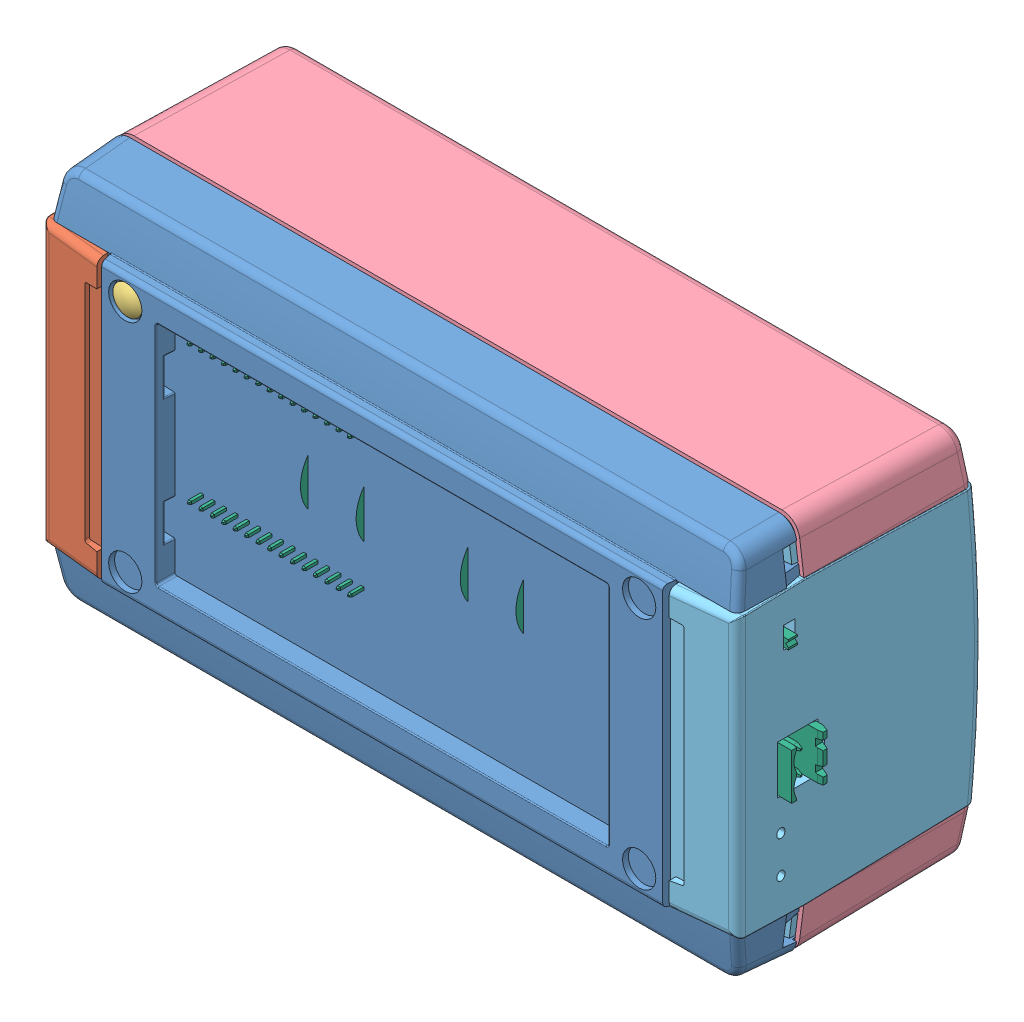
SolidWorks assembly Assembly, configuration Default. Lengths in mm.
Overall size (160.27 84 56.92).
19 component instances, 12 part files, 12 mates.
Components (placement in the parent):
- B1060365 154_84_56-1: B1060365 154_84_56 [Default] at (1.25 0 -12.8) x (0 1 0) z (-1 0 0) size (84 72.92 156.75)
  - 00007483 - 154 Unterteil-1: 00007483 - 154 Unterteil [Default] x (-1 0 0) z (0 0 -1) size (84 17.8 153.5)
  - 00007882 - Gummifuss  D6,5 x 2 mm-1: 00007882 - Gummifuss  D6,5 x 2 mm [Default] at (26 -15.6 -57) x (0.536953 0 0.843612) z (0.843612 0 -0.536953) size (6.6 2.04 6.75) (hidden)
  - 00006113 - 154 Stirnteil H ohne Lⁿftung-5: 00006113 - 154 Stirnteil H ohne Lⁿftung [Default] at (0 -16.8 63.3) x (0 0 1) z (-1 0 0) size (15.5 56 77)
  - 00007882 - Gummifuss  D6,5 x 2 mm-2: 00007882 - Gummifuss  D6,5 x 2 mm [Default] at (26 -15.6 57) x (0.536953 0 0.843612) z (0.843612 0 -0.536953) size (6.6 2.04 6.75)
  - 00007882 - Gummifuss  D6,5 x 2 mm-3: 00007882 - Gummifuss  D6,5 x 2 mm [Default] at (-26 -15.6 57) x (-0.536953 0 -0.843612) z (-0.843612 0 0.536953) size (6.6 2.04 6.75) (hidden)
  - 00006613 - Wandhalter 154_Default-1: 00006613 - Wandhalter 154_Default [Default] at (0 -12.8 1.25) x (0 0 -1) z (0 -1 0) size (133 49.6 8) (hidden)
  - 00007733 - Rastfuss-1: 00007733 - Rastfuss [Default] at (0 -15 38) x (-1 0 0) z (0 0 1) size (11.01 20.6 76) (hidden)
  - 00007864 - Liko-Schraube 2.5x6 Arnold Plastide 45 KS Z (PZ1) blau verz.-1: 00007864 - Liko-Schraube 2.5x6 Arnold Plastide 45 KS Z (PZ1) blau verz. [Default] at (-31.5 -4.7 -58) size (4 7.8 4) (hidden)
  - 00007864 - Liko-Schraube 2.5x6 Arnold Plastide 45 KS Z (PZ1) blau verz.-2: 00007864 - Liko-Schraube 2.5x6 Arnold Plastide 45 KS Z (PZ1) blau verz. [Default] at (29 -4.7 58) x (-1 0 0) z (0 0 -1) size (4 7.8 4) (hidden)
  - 00007864 - Liko-Schraube 2.5x6 Arnold Plastide 45 KS Z (PZ1) blau verz.-3: 00007864 - Liko-Schraube 2.5x6 Arnold Plastide 45 KS Z (PZ1) blau verz. [Default] at (-29 -4.7 58) size (4 7.8 4) (hidden)
  - 00007864 - Liko-Schraube 2.5x6 Arnold Plastide 45 KS Z (PZ1) blau verz.-4: 00007864 - Liko-Schraube 2.5x6 Arnold Plastide 45 KS Z (PZ1) blau verz. [Default] at (31.5 -4.7 -58) x (-1 0 0) z (0 0 -1) size (4 7.8 4) (hidden)
  - 00007482 - 154 Oberteil H-1: 00007482 - 154 Oberteil H [Default] at origin size (84 37.76 153.73)
  - 00007882 - Gummifuss  D6,5 x 2 mm-4: 00007882 - Gummifuss  D6,5 x 2 mm [Default] at (-26 -15.6 -57) x (-0.536953 0 -0.843612) z (-0.843612 0 0.536953) size (6.6 2.04 6.75) (hidden)
  - 00006113 - 156 Stirnteil H ohne Lⁿftung-1: 00006113 - 156 Stirnteil H ohne Lⁿftung [Default] at (0 -16.4764 -63.3454) x (0 0 -1) z (1 0 0) size (15.5 56 77)
- PCB5_Altuim-1: PCB5_Altuim [Default] at (-71.752 -153.051 -18.1194) x (0 1 0) z (0 0 -1) size (75.03 156.42 35.06) (hidden)
- PCB6_Altuim-1: PCB6_Altuim [Default] at (-100.403 -65.036 -16.9115) x (0 1 0) z (0 0 -1) size (75.18 156.42 35.06) (hidden)
- PCB_Voltix_v8.4-1: PCB_Voltix_v8.4 [Défaut] at (-99.49 -65.036 -6.9115) x (0 1 0) z (0 0 -1) size (75.16 160.27 34.6)
- Ledss-1: Ledss [Défaut] at (51.0563 -24.9243 -6.9115) x (0 1 0) z (0 0 -1) size (4 11.76 39.59)
Mates (geometry in assembly coordinates):
- Coincident1: coordinate: point of B1060365 154_84_56-1/00006613 - Wandhalter 154_Default-1; point of assembly
- Concentric12: concentric anti-aligned: cylinder of B1060365 154_84_56-1/00007864 - Liko-Schraube 2.5x6 Arnold Plastide 45 KS Z (PZ1) blau verz.-4 through (59.25 31.5 -2.1) axis (0 0 -1) radius 1.25; cylinder of PCB5_Altuim-1 through (59.25 31.5 -16.5) axis (0 0 1) radius 1.5
- Parallel6: parallel anti-aligned: plane of B1060365 154_84_56-1/00006113 - 156 Stirnteil H ohne Lⁿftung-1 through (75.7954 0 247.6764) normal (-1 0 0); plane of PCB5_Altuim-1 through (74.704 -13.726 -16.5) normal (1 0 0)
- Distance3: distance = 10 mm anti-aligned: plane of B1060365 154_84_56-1/00007483 - 154 Unterteil-1 through (59.25 31.5 -6.5) normal (0 0 -1); plane of PCB6_Altuim-1 through (1.2255 -0.1709 -16.5) normal (0 0 1)
- Concentric13: concentric anti-aligned: cylinder of B1060365 154_84_56-1/00007864 - Liko-Schraube 2.5x6 Arnold Plastide 45 KS Z (PZ1) blau verz.-4 through (59.25 31.5 -2.1) axis (0 0 -1) radius 1.25; cylinder of PCB6_Altuim-1 through (59.25 31.5 -16.5) axis (0 0 1) radius 1.5
- Parallel7: parallel anti-aligned: plane of B1060365 154_84_56-1/00006113 - 156 Stirnteil H ohne Lⁿftung-1 through (75.7954 0 247.6764) normal (-1 0 0); plane of PCB6_Altuim-1 through (74.73 -13.243 -16.5) normal (1 0 0)
- Distance4: distance = 0 mm anti-aligned: plane of B1060365 154_84_56-1/00007483 - 154 Unterteil-1 through (-56.75 29 -6.5) normal (0 0 -1); plane of PCB_Voltix_v8.4-1 through (1.2185 -0.1501 -6.5) normal (0 0 1)
- Parallèle1: parallel anti-aligned: plane of B1060365 154_84_56-1/00006113 - 156 Stirnteil H ohne Lⁿftung-1 through (75.7954 0 247.6764) normal (-1 0 0); plane of PCB_Voltix_v8.4-1 through (74.73 -13.144 -6.5) normal (1 0 0)
- Coaxiale1: concentric anti-aligned: cylinder of B1060365 154_84_56-1/00007864 - Liko-Schraube 2.5x6 Arnold Plastide 45 KS Z (PZ1) blau verz.-4 through (59.25 31.5 -2.1) axis (0 0 -1) radius 1.25; cylinder of PCB_Voltix_v8.4-1 through (59.25 31.5 -6.5) axis (0 0 1) radius 1.5
- Coïncidente1: coincident anti-aligned: plane of PCB_Voltix_v8.4-1 through (1.2185 -0.1501 -6.9115) normal (0 0 -1); plane of Ledss-1 through (51.0563 -24.9243 -6.9115) normal (0 0 1)
- Coaxiale2: concentric aligned: circle of PCB_Voltix_v8.4-1; cylinder of Ledss-1 through (47.1743 -24.9243 -52.1569) axis (0 0 1) radius 1.5
- Parallèle3: parallel aligned: plane of PCB_Voltix_v8.4-1 through (-65.3 -37.731 -6.5) normal (0 -1 0); plane of Ledss-1 through (51.0563 -25.9243 -26.9115) normal (0 -1 0)
